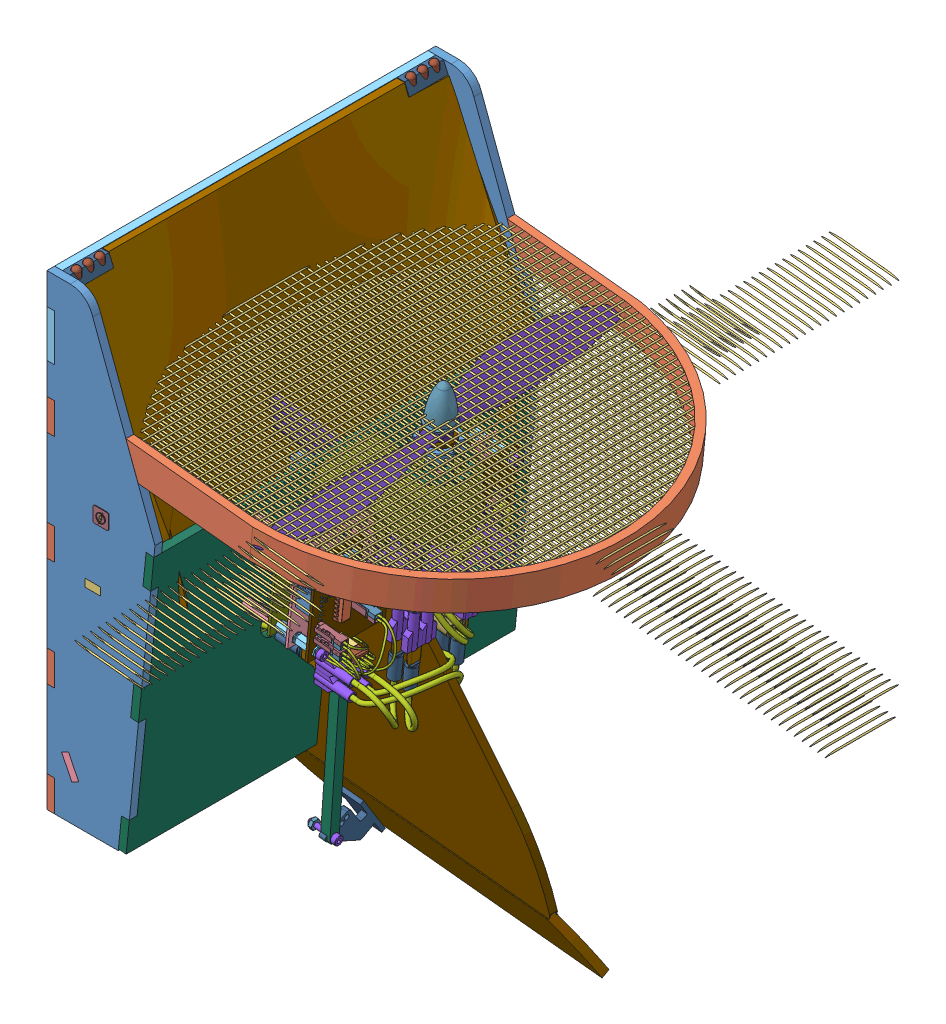
SolidWorks assembly AssTotaleSimu, configuration Défaut. Lengths in mm. (continued)
Components (placement in the parent): (continued)
- AssStructSimu-1: AssStructSimu [Défaut] at (-125.7658 -1.8483 624.6548) x (1 0 0) z (0 0 -1) size (323.53 326.04 251.6) (continued)
  - AssProtec-1: AssProtec [Défaut] at (86.6746 190.4649 284.6351) x (0 0 -1) z (0.101852 -0.9948 0) size (250 237.46 20) (continued)
    - AssGrillage-2: AssGrillage [Défaut] at (339.6086 -132.5428 241.6839) x (0 0 1) z (-1 0 0) size (2.02 237.05 250) (continued)
      - barreau-208: barreau [Défaut] at (-0.1839 -1.5314 233.7823) x (0.998922 0 0.04641) z (0 1 0) size (1 1 400)
      - barreau-209: barreau [Défaut] at (-0.1839 -1.5314 228.7823) x (0.998922 0 0.04641) z (0 1 0) size (1 1 400)
      - barreau-210: barreau [Défaut] at (-0.1839 -1.5314 223.7823) x (0.998922 0 0.04641) z (0 1 0) size (1 1 400)
      - barreau-211: barreau [Défaut] at (-0.1839 -1.5314 218.7823) x (0.998922 0 0.04641) z (0 1 0) size (1 1 400)
      - barreau-212: barreau [Défaut] at (-0.1839 -1.5314 213.7823) x (0.998922 0 0.04641) z (0 1 0) size (1 1 400)
      - barreau-213: barreau [Défaut] at (-0.1839 -1.5314 208.7823) x (0.998922 0 0.04641) z (0 1 0) size (1 1 400)
      - barreau-214: barreau [Défaut] at (-0.1839 -1.5314 203.7823) x (0.998922 0 0.04641) z (0 1 0) size (1 1 400)
  - AssCarte-1: AssCarte [Défaut] at (-42.8534 32.2132 302.028) x (-0.101852 0.9948 0) z (0.9948 0.101852 0) size (91.19 130.57 98.45)
    - carte_onduleur_v4-1: carte_onduleur_v4 [Défaut] at (-25.7639 0.8332 112.9379) size (66.52 130.57 82.34)
      - Layer_1-1: Layer_1 [Défaut] at origin size (60 130 1.61)
      - BTN-1: BTN [Défaut] at (-25.5 7.4 0.803) x (0 -1 0) z (0 0 1) size (6.76 3.64 4.37)
        - Open CASCADE STEP translator 6.8 1.2.1-1: Open CASCADE STEP translator 6.8 1.2.1 [Défaut] at origin size (6.76 3.64 4.37)
          - Body_1-1: Body_1 [Défaut] at (-0.5 -2 0) size (6.76 3.64 4.37)
            - =_[0_1_1_3]-1: =_[0_1_1_3] [Défaut] at origin size (6 3.64 4.37)
            - =_[0_1_1_4]-1: =_[0_1_1_4] [Défaut] at origin size (0.38 1 0.67)
            - =_[0_1_1_5]-1: =_[0_1_1_5] [Défaut] at origin size (0.38 1 0.67)
      - CON_IO1-1: CON_IO1 [Défaut] at (-11.3 12.1 0.803) x (0 -1 0) z (0 0 1) size (16.74 30.7 57.5)
        - Open CASCADE STEP translator 6.8 1.3.1-1: Open CASCADE STEP translator 6.8 1.3.1 [Défaut] at origin size (16.74 30.7 57.5)
          - Body_1_2-1: Body_1_2 [Défaut] at (-3 -15 8) x (0 -1 0) z (-1 0 0) size (30.7 57.5 16.74)
            - 1-1: 1 [Défaut] at origin size (30 50 1.61)
            - 10-1: 10 [Défaut] at (-14.395 31.0465 0.803) x (-1 0 0) z (0 0 1) size (5.59 6.35 1.11)
              - =_[0_1_1_4]-1: =_[0_1_1_4] [Défaut] at origin size (5.59 6.35 1.11)
                - 11-1: 11 [Défaut] at (2 3.3 0) x (-1 0 0) z (0 0 1) size (5.59 6.35 1.11)
                  - =_[0_1_1_3]_2-1: =_[0_1_1_3]_2 [Défaut] at origin size (0.44 0.55 0.36)
                  - =_[0_1_1_4]_2-1: =_[0_1_1_4]_2 [Défaut] at origin size (5.59 4.15 0.36)
                  - =_[0_1_1_5]_2-1: =_[0_1_1_5]_2 [Défaut] at origin size (5.35 6.1 1.1)
                  - =_[0_1_1_6]-1: =_[0_1_1_6] [Défaut] at origin size (0.44 0.55 0.36)
                  - =_[0_1_1_7]-1: =_[0_1_1_7] [Défaut] at origin size (0.44 0.55 0.36)
                  - =_[0_1_1_8]-1: =_[0_1_1_8] [Défaut] at origin size (0.44 0.55 0.36)
            - 13-1: 13 [Défaut] at (-12.62 16.6 -0.803) x (-1 0 0) z (0 0 -1) size (5.59 6.35 1.11)
              - =_[0_1_1_13]-1: =_[0_1_1_13] [Défaut] at origin size (5.59 6.35 1.11)
                - 11-1: 11 [Défaut] at (2 3.3 0) x (-1 0 0) z (0 0 1) size (5.59 6.35 1.11)
                  - =_[0_1_1_3]_2-1: =_[0_1_1_3]_2 [Défaut] at origin size (0.44 0.55 0.36)
                  - =_[0_1_1_4]_2-1: =_[0_1_1_4]_2 [Défaut] at origin size (5.59 4.15 0.36)
                  - =_[0_1_1_5]_2-1: =_[0_1_1_5]_2 [Défaut] at origin size (5.35 6.1 1.1)
                  - =_[0_1_1_6]-1: =_[0_1_1_6] [Défaut] at origin size (0.44 0.55 0.36)
                  - =_[0_1_1_7]-1: =_[0_1_1_7] [Défaut] at origin size (0.44 0.55 0.36)
                  - =_[0_1_1_8]-1: =_[0_1_1_8] [Défaut] at origin size (0.44 0.55 0.36)
            - 16-1: 16 [Défaut] at (-4.2 24.2 0.803) x (-1 0 0) z (0 0 1) size (12.8 0.5 13)
              - =_[0_1_1_15]-1: =_[0_1_1_15] [Défaut] at origin size (12.8 0.5 13)
                - 17-1: 17 [Défaut] at (2.7 0 0) x (1 0 0) z (0 -1 0) size (12.8 13 0.5)
            - 19-1: 19 [Défaut] at (-4.1 6.8 0.803) x (-1 0 0) z (0 0 1) size (12.8 0.5 13)
              - =_[0_1_1_18]-1: =_[0_1_1_18] [Défaut] at origin size (12.8 0.5 13)
                - 17-1: 17 [Défaut] at (2.7 0 0) x (1 0 0) z (0 -1 0) size (12.8 13 0.5)
            - 24-1: 24 [Défaut] at (-8.1 16.5 -0.803) x (0 1 0) z (0 0 -1) size (7.75 5.13 1.17)
              - =_[0_1_1_20]-1: =_[0_1_1_20] [Défaut] at origin size (7.75 5.13 1.17)
                - 20-1: 20 [Défaut] at origin size (7.59 5.13 1.07)
                - 21-1: 21 [Défaut] at (-14.478 0 0) x (-1 0 0) z (0 0 1) size (0.76 5.08 1.17)
                - 22-1: 22 [Défaut] at origin size (0.76 5.08 1.17)
            - 35-1: 35 [Défaut] at (-25.3 25.5 0.803) x (0 -1 0) z (0 0 1) size (6.05 5.2 1.7)
              - =_[0_1_1_25]-1: =_[0_1_1_25] [Défaut] at origin size (6.05 5.2 1.7)
                - 25-1: 25 [Défaut] at origin size (4.3 5.2 1.53)
                - 26-1: 26 [Défaut] at origin size (0.88 0.51 1.06)
                - 27-1: 27 [Défaut] at origin size (0.88 0.51 1.06)
                - 28-1: 28 [Défaut] at origin size (0.88 0.51 1.06)
                - 29-1: 29 [Défaut] at origin size (0.88 0.51 1.06)
                - 30-1: 30 [Défaut] at (11.6 -5.08 0) x (-1 0 0) z (0 0 1) size (0.87 0.51 1.06)
                - 31-1: 31 [Défaut] at (11.6 -2.54 0) x (-1 0 0) z (0 0 1) size (0.87 0.51 1.06)
                - 32-1: 32 [Défaut] at (11.6 0 0) x (-1 0 0) z (0 0 1) size (0.87 0.51 1.06)
                - 33-1: 33 [Défaut] at (11.6 2.54 0) x (-1 0 0) z (0 0 1) size (0.87 0.51 1.06)
            - 40-1: 40 [Défaut] at (-27.6 27.2 0.803) size (2.34 1.04 0.5)
              - =_[0_1_1_36]-1: =_[0_1_1_36] [Défaut] at origin size (2.34 1.04 0.5)
                - 36-1: 36 [Défaut] at origin size (2.29 1.04 0.43)
                - 37-1: 37 [Défaut] at (0.3048 0 0) x (-1 0 0) z (0 0 1) size (0.51 1.02 0.5)
                - 38-1: 38 [Défaut] at origin size (0.51 1.02 0.5)
            - 42-1: 42 [Défaut] at (-22.1 21.6 0.803) x (0 1 0) z (0 0 1) size (2.34 1.04 0.5)
              - =_[0_1_1_36]-1: =_[0_1_1_36] [Défaut] at origin size (2.34 1.04 0.5)
                - 36-1: 36 [Défaut] at origin size (2.29 1.04 0.43)
                - 37-1: 37 [Défaut] at (0.3048 0 0) x (-1 0 0) z (0 0 1) size (0.51 1.02 0.5)
                - 38-1: 38 [Défaut] at origin size (0.51 1.02 0.5)
            - 47-1: 47 [Défaut] at (-14.7664 14.5 -0.803) x (-1 0 0) z (0 0 -1) size (2.34 1.04 0.5)
              - =_[0_1_1_42]-1: =_[0_1_1_42] [Défaut] at origin size (2.34 1.04 0.5)
                - 43-1: 43 [Défaut] at origin size (2.29 1.04 0.43)
                - 44-1: 44 [Défaut] at (0.3048 0 0) x (-1 0 0) z (0 0 1) size (0.51 1.02 0.5)
                - 45-1: 45 [Défaut] at origin size (0.51 1.02 0.5)
            - 57-1: 57 [Défaut] at (-15.3 2.7 -0.803) x (0 -1 0) z (0 0 -1) size (10.36 15.24 6.14)
              - =_[0_1_1_47]-1: =_[0_1_1_47] [Défaut] at origin size (10.36 15.24 6.14)
                - 55-1: 55 [Défaut] at (1.8 -1.2 3) x (1 0 0) z (0 1 0) size (10.36 6.14 15.24)
                  - 54-1: 54 [Défaut] at origin size (10.36 6.14 7.62)
                    - 52-1: 52 [Défaut] at origin size (10.36 6.14 2.54)
                      - 48-1: 48 [Défaut] at origin size (8.4 2.54 2.54)
                      - 49-1: 49 [Défaut] at (-0.0461 1.2682 1.27) x (0 0 -1) z (0.999998 -0.002105 0) size (1.95 5.07 7.58)
                    - 52-2: 52 [Défaut] at (0 0 -2.54) size (10.36 6.14 2.54)
                      - 48-1: 48 [Défaut] at origin size (8.4 2.54 2.54)
                      - 49-1: 49 [Défaut] at (-0.0461 1.2682 1.27) x (0 0 -1) z (0.999998 -0.002105 0) size (1.95 5.07 7.58)
                    - 52-3: 52 [Défaut] at (0 0 -5.08) size (10.36 6.14 2.54)
                      - 48-1: 48 [Défaut] at origin size (8.4 2.54 2.54)
                      - 49-1: 49 [Défaut] at (-0.0461 1.2682 1.27) x (0 0 -1) z (0.999998 -0.002105 0) size (1.95 5.07 7.58)
                  - 54-2: 54 [Défaut] at (0 0 -7.62) size (10.36 6.14 7.62)
                    - 52-1: 52 [Défaut] at origin size (10.36 6.14 2.54)
                      - 48-1: 48 [Défaut] at origin size (8.4 2.54 2.54)
                      - 49-1: 49 [Défaut] at (-0.0461 1.2682 1.27) x (0 0 -1) z (0.999998 -0.002105 0) size (1.95 5.07 7.58)
                    - 52-2: 52 [Défaut] at (0 0 -2.54) size (10.36 6.14 2.54)
                      - 48-1: 48 [Défaut] at origin size (8.4 2.54 2.54)
                      - 49-1: 49 [Défaut] at (-0.0461 1.2682 1.27) x (0 0 -1) z (0.999998 -0.002105 0) size (1.95 5.07 7.58)
                    - 52-3: 52 [Défaut] at (0 0 -5.08) size (10.36 6.14 2.54)
                      - 48-1: 48 [Défaut] at origin size (8.4 2.54 2.54)
                      - 49-1: 49 [Défaut] at (-0.0461 1.2682 1.27) x (0 0 -1) z (0.999998 -0.002105 0) size (1.95 5.07 7.58)
            - 59-1: 59 [Défaut] at (-26.5 31 0.803) x (0 -1 0) z (0 0 1) size (2.34 1.04 0.5)
              - =_[0_1_1_42]-1: =_[0_1_1_42] [Défaut] at origin size (2.34 1.04 0.5)
                - 43-1: 43 [Défaut] at origin size (2.29 1.04 0.43)
                - 44-1: 44 [Défaut] at (0.3048 0 0) x (-1 0 0) z (0 0 1) size (0.51 1.02 0.5)
                - 45-1: 45 [Défaut] at origin size (0.51 1.02 0.5)
            - 61-1: 61 [Défaut] at (-21.6 17.8 0.803) x (-1 0 0) z (0 0 1) size (2.34 1.04 0.5)
              - =_[0_1_1_42]-1: =_[0_1_1_42] [Défaut] at origin size (2.34 1.04 0.5)
                - 43-1: 43 [Défaut] at origin size (2.29 1.04 0.43)
                - 44-1: 44 [Défaut] at (0.3048 0 0) x (-1 0 0) z (0 0 1) size (0.51 1.02 0.5)
                - 45-1: 45 [Défaut] at origin size (0.51 1.02 0.5)
            - 64-1: 64 [Défaut] at (-3.3 17.6 0.803) x (0 -1 0) z (0 0 1) size (8.01 8 14.24)
              - =_[0_1_1_56]-1: =_[0_1_1_56] [Défaut] at origin size (8.01 8 14.24)
                - 62-1: 62 [Défaut] at (1.8 0 0) x (1 0 0) z (0 -1 0) size (8.01 14.24 8)
      - CON_IO2-1: CON_IO2 [Défaut] at (-11.3 -2.7 0.803) x (0 -1 0) z (0 0 1) size (16.74 30.7 57.5)
        - Open CASCADE STEP translator 6.8 1.4.1-1: Open CASCADE STEP translator 6.8 1.4.1 [Défaut] at origin size (16.74 30.7 57.5)
          - Body_1_2-1: Body_1_2 [Défaut] at (-3 -15 8) x (0 -1 0) z (-1 0 0) size (30.7 57.5 16.74)
            - 1-1: 1 [Défaut] at origin size (30 50 1.61)
            - 10-1: 10 [Défaut] at (-14.395 31.0465 0.803) x (-1 0 0) z (0 0 1) size (5.59 6.35 1.11)
              - =_[0_1_1_4]-1: =_[0_1_1_4] [Défaut] at origin size (5.59 6.35 1.11)
                - 11-1: 11 [Défaut] at (2 3.3 0) x (-1 0 0) z (0 0 1) size (5.59 6.35 1.11)
                  - =_[0_1_1_3]_2-1: =_[0_1_1_3]_2 [Défaut] at origin size (0.44 0.55 0.36)
                  - =_[0_1_1_4]_2-1: =_[0_1_1_4]_2 [Défaut] at origin size (5.59 4.15 0.36)
                  - =_[0_1_1_5]_2-1: =_[0_1_1_5]_2 [Défaut] at origin size (5.35 6.1 1.1)
                  - =_[0_1_1_6]-1: =_[0_1_1_6] [Défaut] at origin size (0.44 0.55 0.36)
                  - =_[0_1_1_7]-1: =_[0_1_1_7] [Défaut] at origin size (0.44 0.55 0.36)
                  - =_[0_1_1_8]-1: =_[0_1_1_8] [Défaut] at origin size (0.44 0.55 0.36)
            - 13-1: 13 [Défaut] at (-12.62 16.6 -0.803) x (-1 0 0) z (0 0 -1) size (5.59 6.35 1.11)
              - =_[0_1_1_13]-1: =_[0_1_1_13] [Défaut] at origin size (5.59 6.35 1.11)
                - 11-1: 11 [Défaut] at (2 3.3 0) x (-1 0 0) z (0 0 1) size (5.59 6.35 1.11)
                  - =_[0_1_1_3]_2-1: =_[0_1_1_3]_2 [Défaut] at origin size (0.44 0.55 0.36)
                  - =_[0_1_1_4]_2-1: =_[0_1_1_4]_2 [Défaut] at origin size (5.59 4.15 0.36)
                  - =_[0_1_1_5]_2-1: =_[0_1_1_5]_2 [Défaut] at origin size (5.35 6.1 1.1)
                  - =_[0_1_1_6]-1: =_[0_1_1_6] [Défaut] at origin size (0.44 0.55 0.36)
                  - =_[0_1_1_7]-1: =_[0_1_1_7] [Défaut] at origin size (0.44 0.55 0.36)
                  - =_[0_1_1_8]-1: =_[0_1_1_8] [Défaut] at origin size (0.44 0.55 0.36)
            - 16-1: 16 [Défaut] at (-4.2 24.2 0.803) x (-1 0 0) z (0 0 1) size (12.8 0.5 13)
              - =_[0_1_1_15]-1: =_[0_1_1_15] [Défaut] at origin size (12.8 0.5 13)
                - 17-1: 17 [Défaut] at (2.7 0 0) x (1 0 0) z (0 -1 0) size (12.8 13 0.5)
            - 19-1: 19 [Défaut] at (-4.1 6.8 0.803) x (-1 0 0) z (0 0 1) size (12.8 0.5 13)
              - =_[0_1_1_18]-1: =_[0_1_1_18] [Défaut] at origin size (12.8 0.5 13)
                - 17-1: 17 [Défaut] at (2.7 0 0) x (1 0 0) z (0 -1 0) size (12.8 13 0.5)
            - 24-1: 24 [Défaut] at (-8.1 16.5 -0.803) x (0 1 0) z (0 0 -1) size (7.75 5.13 1.17)
              - =_[0_1_1_20]-1: =_[0_1_1_20] [Défaut] at origin size (7.75 5.13 1.17)
                - 20-1: 20 [Défaut] at origin size (7.59 5.13 1.07)
                - 21-1: 21 [Défaut] at (-14.478 0 0) x (-1 0 0) z (0 0 1) size (0.76 5.08 1.17)
                - 22-1: 22 [Défaut] at origin size (0.76 5.08 1.17)
            - 35-1: 35 [Défaut] at (-25.3 25.5 0.803) x (0 -1 0) z (0 0 1) size (6.05 5.2 1.7)
              - =_[0_1_1_25]-1: =_[0_1_1_25] [Défaut] at origin size (6.05 5.2 1.7)
                - 25-1: 25 [Défaut] at origin size (4.3 5.2 1.53)
                - 26-1: 26 [Défaut] at origin size (0.88 0.51 1.06)
                - 27-1: 27 [Défaut] at origin size (0.88 0.51 1.06)
                - 28-1: 28 [Défaut] at origin size (0.88 0.51 1.06)
                - 29-1: 29 [Défaut] at origin size (0.88 0.51 1.06)
                - 30-1: 30 [Défaut] at (11.6 -5.08 0) x (-1 0 0) z (0 0 1) size (0.87 0.51 1.06)
                - 31-1: 31 [Défaut] at (11.6 -2.54 0) x (-1 0 0) z (0 0 1) size (0.87 0.51 1.06)
                - 32-1: 32 [Défaut] at (11.6 0 0) x (-1 0 0) z (0 0 1) size (0.87 0.51 1.06)
                - 33-1: 33 [Défaut] at (11.6 2.54 0) x (-1 0 0) z (0 0 1) size (0.87 0.51 1.06)
            - 40-1: 40 [Défaut] at (-27.6 27.2 0.803) size (2.34 1.04 0.5)
              - =_[0_1_1_36]-1: =_[0_1_1_36] [Défaut] at origin size (2.34 1.04 0.5)
                - 36-1: 36 [Défaut] at origin size (2.29 1.04 0.43)
                - 37-1: 37 [Défaut] at (0.3048 0 0) x (-1 0 0) z (0 0 1) size (0.51 1.02 0.5)
                - 38-1: 38 [Défaut] at origin size (0.51 1.02 0.5)
            - 42-1: 42 [Défaut] at (-22.1 21.6 0.803) x (0 1 0) z (0 0 1) size (2.34 1.04 0.5)
              - =_[0_1_1_36]-1: =_[0_1_1_36] [Défaut] at origin size (2.34 1.04 0.5)
                - 36-1: 36 [Défaut] at origin size (2.29 1.04 0.43)
                - 37-1: 37 [Défaut] at (0.3048 0 0) x (-1 0 0) z (0 0 1) size (0.51 1.02 0.5)
                - 38-1: 38 [Défaut] at origin size (0.51 1.02 0.5)
            - 47-1: 47 [Défaut] at (-14.7664 14.5 -0.803) x (-1 0 0) z (0 0 -1) size (2.34 1.04 0.5)
              - =_[0_1_1_42]-1: =_[0_1_1_42] [Défaut] at origin size (2.34 1.04 0.5)
                - 43-1: 43 [Défaut] at origin size (2.29 1.04 0.43)
                - 44-1: 44 [Défaut] at (0.3048 0 0) x (-1 0 0) z (0 0 1) size (0.51 1.02 0.5)
                - 45-1: 45 [Défaut] at origin size (0.51 1.02 0.5)
            - 57-1: 57 [Défaut] at (-15.3 2.7 -0.803) x (0 -1 0) z (0 0 -1) size (10.36 15.24 6.14)
              - =_[0_1_1_47]-1: =_[0_1_1_47] [Défaut] at origin size (10.36 15.24 6.14)
                - 55-1: 55 [Défaut] at (1.8 -1.2 3) x (1 0 0) z (0 1 0) size (10.36 6.14 15.24)
                  - 54-1: 54 [Défaut] at origin size (10.36 6.14 7.62)
                    - 52-1: 52 [Défaut] at origin size (10.36 6.14 2.54)
                      - 48-1: 48 [Défaut] at origin size (8.4 2.54 2.54)
                      - 49-1: 49 [Défaut] at (-0.0461 1.2682 1.27) x (0 0 -1) z (0.999998 -0.002105 0) size (1.95 5.07 7.58)
                    - 52-2: 52 [Défaut] at (0 0 -2.54) size (10.36 6.14 2.54)
                      - 48-1: 48 [Défaut] at origin size (8.4 2.54 2.54)
                      - 49-1: 49 [Défaut] at (-0.0461 1.2682 1.27) x (0 0 -1) z (0.999998 -0.002105 0) size (1.95 5.07 7.58)
                    - 52-3: 52 [Défaut] at (0 0 -5.08) size (10.36 6.14 2.54)
                      - 48-1: 48 [Défaut] at origin size (8.4 2.54 2.54)
                      - 49-1: 49 [Défaut] at (-0.0461 1.2682 1.27) x (0 0 -1) z (0.999998 -0.002105 0) size (1.95 5.07 7.58)
                  - 54-2: 54 [Défaut] at (0 0 -7.62) size (10.36 6.14 7.62)
                    - 52-1: 52 [Défaut] at origin size (10.36 6.14 2.54)
                      - 48-1: 48 [Défaut] at origin size (8.4 2.54 2.54)
                      - 49-1: 49 [Défaut] at (-0.0461 1.2682 1.27) x (0 0 -1) z (0.999998 -0.002105 0) size (1.95 5.07 7.58)
                    - 52-2: 52 [Défaut] at (0 0 -2.54) size (10.36 6.14 2.54)
                      - 48-1: 48 [Défaut] at origin size (8.4 2.54 2.54)
                      - 49-1: 49 [Défaut] at (-0.0461 1.2682 1.27) x (0 0 -1) z (0.999998 -0.002105 0) size (1.95 5.07 7.58)
                    - 52-3: 52 [Défaut] at (0 0 -5.08) size (10.36 6.14 2.54)
                      - 48-1: 48 [Défaut] at origin size (8.4 2.54 2.54)
                      - 49-1: 49 [Défaut] at (-0.0461 1.2682 1.27) x (0 0 -1) z (0.999998 -0.002105 0) size (1.95 5.07 7.58)
            - 59-1: 59 [Défaut] at (-26.5 31 0.803) x (0 -1 0) z (0 0 1) size (2.34 1.04 0.5)
              - =_[0_1_1_42]-1: =_[0_1_1_42] [Défaut] at origin size (2.34 1.04 0.5)
                - 43-1: 43 [Défaut] at origin size (2.29 1.04 0.43)
                - 44-1: 44 [Défaut] at (0.3048 0 0) x (-1 0 0) z (0 0 1) size (0.51 1.02 0.5)
                - 45-1: 45 [Défaut] at origin size (0.51 1.02 0.5)
            - 61-1: 61 [Défaut] at (-21.6 17.8 0.803) x (-1 0 0) z (0 0 1) size (2.34 1.04 0.5)
              - =_[0_1_1_42]-1: =_[0_1_1_42] [Défaut] at origin size (2.34 1.04 0.5)
                - 43-1: 43 [Défaut] at origin size (2.29 1.04 0.43)
                - 44-1: 44 [Défaut] at (0.3048 0 0) x (-1 0 0) z (0 0 1) size (0.51 1.02 0.5)
                - 45-1: 45 [Défaut] at origin size (0.51 1.02 0.5)
            - 64-1: 64 [Défaut] at (-3.3 17.6 0.803) x (0 -1 0) z (0 0 1) size (8.01 8 14.24)
              - =_[0_1_1_56]-1: =_[0_1_1_56] [Défaut] at origin size (8.01 8 14.24)
                - 62-1: 62 [Défaut] at (1.8 0 0) x (1 0 0) z (0 -1 0) size (8.01 14.24 8)
      - CON_IO3-1: CON_IO3 [Défaut] at (-11.3 -17.7 0.803) x (0 -1 0) z (0 0 1) size (16.74 30.7 57.5)
        - Open CASCADE STEP translator 6.8 1.5.1-1: Open CASCADE STEP translator 6.8 1.5.1 [Défaut] at origin size (16.74 30.7 57.5)
          - Body_1_2-1: Body_1_2 [Défaut] at (-3 -15 8) x (0 -1 0) z (-1 0 0) size (30.7 57.5 16.74)
            - 1-1: 1 [Défaut] at origin size (30 50 1.61)
            - 10-1: 10 [Défaut] at (-14.395 31.0465 0.803) x (-1 0 0) z (0 0 1) size (5.59 6.35 1.11)
              - =_[0_1_1_4]-1: =_[0_1_1_4] [Défaut] at origin size (5.59 6.35 1.11)
                - 11-1: 11 [Défaut] at (2 3.3 0) x (-1 0 0) z (0 0 1) size (5.59 6.35 1.11)
                  - =_[0_1_1_3]_2-1: =_[0_1_1_3]_2 [Défaut] at origin size (0.44 0.55 0.36)
                  - =_[0_1_1_4]_2-1: =_[0_1_1_4]_2 [Défaut] at origin size (5.59 4.15 0.36)
                  - =_[0_1_1_5]_2-1: =_[0_1_1_5]_2 [Défaut] at origin size (5.35 6.1 1.1)
                  - =_[0_1_1_6]-1: =_[0_1_1_6] [Défaut] at origin size (0.44 0.55 0.36)
                  - =_[0_1_1_7]-1: =_[0_1_1_7] [Défaut] at origin size (0.44 0.55 0.36)
                  - =_[0_1_1_8]-1: =_[0_1_1_8] [Défaut] at origin size (0.44 0.55 0.36)
            - 13-1: 13 [Défaut] at (-12.62 16.6 -0.803) x (-1 0 0) z (0 0 -1) size (5.59 6.35 1.11)
              - =_[0_1_1_13]-1: =_[0_1_1_13] [Défaut] at origin size (5.59 6.35 1.11)
                - 11-1: 11 [Défaut] at (2 3.3 0) x (-1 0 0) z (0 0 1) size (5.59 6.35 1.11)
                  - =_[0_1_1_3]_2-1: =_[0_1_1_3]_2 [Défaut] at origin size (0.44 0.55 0.36)
                  - =_[0_1_1_4]_2-1: =_[0_1_1_4]_2 [Défaut] at origin size (5.59 4.15 0.36)
                  - =_[0_1_1_5]_2-1: =_[0_1_1_5]_2 [Défaut] at origin size (5.35 6.1 1.1)
                  - =_[0_1_1_6]-1: =_[0_1_1_6] [Défaut] at origin size (0.44 0.55 0.36)
                  - =_[0_1_1_7]-1: =_[0_1_1_7] [Défaut] at origin size (0.44 0.55 0.36)
                  - =_[0_1_1_8]-1: =_[0_1_1_8] [Défaut] at origin size (0.44 0.55 0.36)
            - 16-1: 16 [Défaut] at (-4.2 24.2 0.803) x (-1 0 0) z (0 0 1) size (12.8 0.5 13)
              - =_[0_1_1_15]-1: =_[0_1_1_15] [Défaut] at origin size (12.8 0.5 13)
                - 17-1: 17 [Défaut] at (2.7 0 0) x (1 0 0) z (0 -1 0) size (12.8 13 0.5)
            - 19-1: 19 [Défaut] at (-4.1 6.8 0.803) x (-1 0 0) z (0 0 1) size (12.8 0.5 13)
              - =_[0_1_1_18]-1: =_[0_1_1_18] [Défaut] at origin size (12.8 0.5 13)
                - 17-1: 17 [Défaut] at (2.7 0 0) x (1 0 0) z (0 -1 0) size (12.8 13 0.5)
            - 24-1: 24 [Défaut] at (-8.1 16.5 -0.803) x (0 1 0) z (0 0 -1) size (7.75 5.13 1.17)
              - =_[0_1_1_20]-1: =_[0_1_1_20] [Défaut] at origin size (7.75 5.13 1.17)
                - 20-1: 20 [Défaut] at origin size (7.59 5.13 1.07)
                - 21-1: 21 [Défaut] at (-14.478 0 0) x (-1 0 0) z (0 0 1) size (0.76 5.08 1.17)
                - 22-1: 22 [Défaut] at origin size (0.76 5.08 1.17)
            - 35-1: 35 [Défaut] at (-25.3 25.5 0.803) x (0 -1 0) z (0 0 1) size (6.05 5.2 1.7)
              - =_[0_1_1_25]-1: =_[0_1_1_25] [Défaut] at origin size (6.05 5.2 1.7)
                - 25-1: 25 [Défaut] at origin size (4.3 5.2 1.53)
                - 26-1: 26 [Défaut] at origin size (0.88 0.51 1.06)
                - 27-1: 27 [Défaut] at origin size (0.88 0.51 1.06)
                - 28-1: 28 [Défaut] at origin size (0.88 0.51 1.06)
                - 29-1: 29 [Défaut] at origin size (0.88 0.51 1.06)
                - 30-1: 30 [Défaut] at (11.6 -5.08 0) x (-1 0 0) z (0 0 1) size (0.87 0.51 1.06)
                - 31-1: 31 [Défaut] at (11.6 -2.54 0) x (-1 0 0) z (0 0 1) size (0.87 0.51 1.06)
                - 32-1: 32 [Défaut] at (11.6 0 0) x (-1 0 0) z (0 0 1) size (0.87 0.51 1.06)
                - 33-1: 33 [Défaut] at (11.6 2.54 0) x (-1 0 0) z (0 0 1) size (0.87 0.51 1.06)
            - 40-1: 40 [Défaut] at (-27.6 27.2 0.803) size (2.34 1.04 0.5)
              - =_[0_1_1_36]-1: =_[0_1_1_36] [Défaut] at origin size (2.34 1.04 0.5)
                - 36-1: 36 [Défaut] at origin size (2.29 1.04 0.43)
                - 37-1: 37 [Défaut] at (0.3048 0 0) x (-1 0 0) z (0 0 1) size (0.51 1.02 0.5)
                - 38-1: 38 [Défaut] at origin size (0.51 1.02 0.5)
            - 42-1: 42 [Défaut] at (-22.1 21.6 0.803) x (0 1 0) z (0 0 1) size (2.34 1.04 0.5)
              - =_[0_1_1_36]-1: =_[0_1_1_36] [Défaut] at origin size (2.34 1.04 0.5)
                - 36-1: 36 [Défaut] at origin size (2.29 1.04 0.43)
                - 37-1: 37 [Défaut] at (0.3048 0 0) x (-1 0 0) z (0 0 1) size (0.51 1.02 0.5)
                - 38-1: 38 [Défaut] at origin size (0.51 1.02 0.5)
            - 47-1: 47 [Défaut] at (-14.7664 14.5 -0.803) x (-1 0 0) z (0 0 -1) size (2.34 1.04 0.5)
              - =_[0_1_1_42]-1: =_[0_1_1_42] [Défaut] at origin size (2.34 1.04 0.5)
                - 43-1: 43 [Défaut] at origin size (2.29 1.04 0.43)
                - 44-1: 44 [Défaut] at (0.3048 0 0) x (-1 0 0) z (0 0 1) size (0.51 1.02 0.5)
                - 45-1: 45 [Défaut] at origin size (0.51 1.02 0.5)
            - 57-1: 57 [Défaut] at (-15.3 2.7 -0.803) x (0 -1 0) z (0 0 -1) size (10.36 15.24 6.14)
              - =_[0_1_1_47]-1: =_[0_1_1_47] [Défaut] at origin size (10.36 15.24 6.14)
                - 55-1: 55 [Défaut] at (1.8 -1.2 3) x (1 0 0) z (0 1 0) size (10.36 6.14 15.24)
                  - 54-1: 54 [Défaut] at origin size (10.36 6.14 7.62)
                    - 52-1: 52 [Défaut] at origin size (10.36 6.14 2.54)
                      - 48-1: 48 [Défaut] at origin size (8.4 2.54 2.54)
                      - 49-1: 49 [Défaut] at (-0.0461 1.2682 1.27) x (0 0 -1) z (0.999998 -0.002105 0) size (1.95 5.07 7.58)
                    - 52-2: 52 [Défaut] at (0 0 -2.54) size (10.36 6.14 2.54)
                      - 48-1: 48 [Défaut] at origin size (8.4 2.54 2.54)
                      - 49-1: 49 [Défaut] at (-0.0461 1.2682 1.27) x (0 0 -1) z (0.999998 -0.002105 0) size (1.95 5.07 7.58)
                    - 52-3: 52 [Défaut] at (0 0 -5.08) size (10.36 6.14 2.54)
                      - 48-1: 48 [Défaut] at origin size (8.4 2.54 2.54)
                      - 49-1: 49 [Défaut] at (-0.0461 1.2682 1.27) x (0 0 -1) z (0.999998 -0.002105 0) size (1.95 5.07 7.58)
                  - 54-2: 54 [Défaut] at (0 0 -7.62) size (10.36 6.14 7.62)
                    - 52-1: 52 [Défaut] at origin size (10.36 6.14 2.54)
                      - 48-1: 48 [Défaut] at origin size (8.4 2.54 2.54)
                      - 49-1: 49 [Défaut] at (-0.0461 1.2682 1.27) x (0 0 -1) z (0.999998 -0.002105 0) size (1.95 5.07 7.58)
                    - 52-2: 52 [Défaut] at (0 0 -2.54) size (10.36 6.14 2.54)
                      - 48-1: 48 [Défaut] at origin size (8.4 2.54 2.54)
                      - 49-1: 49 [Défaut] at (-0.0461 1.2682 1.27) x (0 0 -1) z (0.999998 -0.002105 0) size (1.95 5.07 7.58)
                    - 52-3: 52 [Défaut] at (0 0 -5.08) size (10.36 6.14 2.54)
                      - 48-1: 48 [Défaut] at origin size (8.4 2.54 2.54)
                      - 49-1: 49 [Défaut] at (-0.0461 1.2682 1.27) x (0 0 -1) z (0.999998 -0.002105 0) size (1.95 5.07 7.58)
            - 59-1: 59 [Défaut] at (-26.5 31 0.803) x (0 -1 0) z (0 0 1) size (2.34 1.04 0.5)
              - =_[0_1_1_42]-1: =_[0_1_1_42] [Défaut] at origin size (2.34 1.04 0.5)
                - 43-1: 43 [Défaut] at origin size (2.29 1.04 0.43)
                - 44-1: 44 [Défaut] at (0.3048 0 0) x (-1 0 0) z (0 0 1) size (0.51 1.02 0.5)
                - 45-1: 45 [Défaut] at origin size (0.51 1.02 0.5)
            - 61-1: 61 [Défaut] at (-21.6 17.8 0.803) x (-1 0 0) z (0 0 1) size (2.34 1.04 0.5)
              - =_[0_1_1_42]-1: =_[0_1_1_42] [Défaut] at origin size (2.34 1.04 0.5)
                - 43-1: 43 [Défaut] at origin size (2.29 1.04 0.43)
                - 44-1: 44 [Défaut] at (0.3048 0 0) x (-1 0 0) z (0 0 1) size (0.51 1.02 0.5)
                - 45-1: 45 [Défaut] at origin size (0.51 1.02 0.5)
            - 64-1: 64 [Défaut] at (-3.3 17.6 0.803) x (0 -1 0) z (0 0 1) size (8.01 8 14.24)
              - =_[0_1_1_56]-1: =_[0_1_1_56] [Défaut] at origin size (8.01 8 14.24)
                - 62-1: 62 [Défaut] at (1.8 0 0) x (1 0 0) z (0 -1 0) size (8.01 14.24 8)
      - C1_1-1: C1_1 [Défaut] at (-20.6336 6.4 -0.803) x (1 0 0) z (0 0 -1) size (2.34 1.04 0.5)
        - Open CASCADE STEP translator 6.8 1.6.1-1: Open CASCADE STEP translator 6.8 1.6.1 [Défaut] at origin size (2.34 1.04 0.5)
          - Body_1-1: Body_1 [Défaut] at origin size (2.29 1.04 0.43)
          - Pin_1-1: Pin_1 [Défaut] at (0.3048 0 0) x (-1 0 0) z (0 0 1) size (0.51 1.02 0.5)
          - Pin_2-1: Pin_2 [Défaut] at origin size (0.51 1.02 0.5)
      - C1_2-1: C1_2 [Défaut] at (-24.2 6.4 -0.803) x (1 0 0) z (0 0 -1) size (2.34 1.04 0.5)
        - Open CASCADE STEP translator 6.8 1.6.1-1: Open CASCADE STEP translator 6.8 1.6.1 [Défaut] at origin size (2.34 1.04 0.5)
          - Body_1-1: Body_1 [Défaut] at origin size (2.29 1.04 0.43)
          - Pin_1-1: Pin_1 [Défaut] at (0.3048 0 0) x (-1 0 0) z (0 0 1) size (0.51 1.02 0.5)
          - Pin_2-1: Pin_2 [Défaut] at origin size (0.51 1.02 0.5)
      - C_F-1: C_F [Défaut] at (-16.2432 4.45 -0.803) x (0 -1 0) z (0 0 -1) size (2.34 1.04 0.5)
        - Open CASCADE STEP translator 6.8 1.6.1-1: Open CASCADE STEP translator 6.8 1.6.1 [Défaut] at origin size (2.34 1.04 0.5)
          - Body_1-1: Body_1 [Défaut] at origin size (2.29 1.04 0.43)
          - Pin_1-1: Pin_1 [Défaut] at (0.3048 0 0) x (-1 0 0) z (0 0 1) size (0.51 1.02 0.5)
          - Pin_2-1: Pin_2 [Défaut] at origin size (0.51 1.02 0.5)
      - D_LED_STATE1-1: D_LED_STATE1 [Défaut] at (-6.8906 -21.6 0.803) size (2.34 1.04 0.5)
        - Open CASCADE STEP translator 6.8 1.6.1-1: Open CASCADE STEP translator 6.8 1.6.1 [Défaut] at origin size (2.34 1.04 0.5)
          - Body_1-1: Body_1 [Défaut] at origin size (2.29 1.04 0.43)
          - Pin_1-1: Pin_1 [Défaut] at (0.3048 0 0) x (-1 0 0) z (0 0 1) size (0.51 1.02 0.5)
          - Pin_2-1: Pin_2 [Défaut] at origin size (0.51 1.02 0.5)
      - PICKIT-1: PICKIT [Défaut] at (-24.1 -30.5 0.803) size (15.24 5 14.3)
        - Open CASCADE STEP translator 6.8 1.10.1-1: Open CASCADE STEP translator 6.8 1.10.1 [Défaut] at origin size (15.24 5 14.3)
          - Body_1_2-1: Body_1_2 [Défaut] at (6.3 0 12) size (15.24 5 14.3)
      - C_DEC_CUR-1: C_DEC_CUR [Défaut] at (-8.9496 5.7572 -0.803) x (0 1 0) z (0 0 -1) size (2.34 1.04 0.5)
        - Open CASCADE STEP translator 6.8 1.6.1-1: Open CASCADE STEP translator 6.8 1.6.1 [Défaut] at origin size (2.34 1.04 0.5)
          - Body_1-1: Body_1 [Défaut] at origin size (2.29 1.04 0.43)
          - Pin_1-1: Pin_1 [Défaut] at (0.3048 0 0) x (-1 0 0) z (0 0 1) size (0.51 1.02 0.5)
          - Pin_2-1: Pin_2 [Défaut] at origin size (0.51 1.02 0.5)
      - R_F-1: R_F [Défaut] at (-14.65 4.4432 -0.803) x (0 -1 0) z (0 0 -1) size (2.34 1.04 0.5)
        - Open CASCADE STEP translator 6.8 1.12.1-1: Open CASCADE STEP translator 6.8 1.12.1 [Défaut] at origin size (2.34 1.04 0.5)
          - Body_1_3-1: Body_1_3 [Défaut] at origin size (2.29 1.04 0.43)
          - Pin_1_2-1: Pin_1_2 [Défaut] at (0.3048 0 0) x (-1 0 0) z (0 0 1) size (0.51 1.02 0.5)
          - Pin_2_2-1: Pin_2_2 [Défaut] at origin size (0.51 1.02 0.5)
      - R_GAIN1-1: R_GAIN1 [Défaut] at (-13.95 5.7568 -0.803) x (0 1 0) z (0 0 -1) size (2.34 1.04 0.5)
        - Open CASCADE STEP translator 6.8 1.12.1-1: Open CASCADE STEP translator 6.8 1.12.1 [Défaut] at origin size (2.34 1.04 0.5)
          - Body_1_3-1: Body_1_3 [Défaut] at origin size (2.29 1.04 0.43)
          - Pin_1_2-1: Pin_1_2 [Défaut] at (0.3048 0 0) x (-1 0 0) z (0 0 1) size (0.51 1.02 0.5)
          - Pin_2_2-1: Pin_2_2 [Défaut] at origin size (0.51 1.02 0.5)
      - R_GAIN2-1: R_GAIN2 [Défaut] at (-15.65 7.9176 -0.803) x (0 -1 0) z (0 0 -1) size (2.34 1.04 0.5)
        - Open CASCADE STEP translator 6.8 1.12.1-1: Open CASCADE STEP translator 6.8 1.12.1 [Défaut] at origin size (2.34 1.04 0.5)
          - Body_1_3-1: Body_1_3 [Défaut] at origin size (2.29 1.04 0.43)
          - Pin_1_2-1: Pin_1_2 [Défaut] at (0.3048 0 0) x (-1 0 0) z (0 0 1) size (0.51 1.02 0.5)
          - Pin_2_2-1: Pin_2_2 [Défaut] at origin size (0.51 1.02 0.5)
      - R_LED_STATE1-1: R_LED_STATE1 [Défaut] at (-6.9242 -19.9 0.803) size (2.34 1.04 0.5)
        - Open CASCADE STEP translator 6.8 1.12.1-1: Open CASCADE STEP translator 6.8 1.12.1 [Défaut] at origin size (2.34 1.04 0.5)
          - Body_1_3-1: Body_1_3 [Défaut] at origin size (2.29 1.04 0.43)
          - Pin_1_2-1: Pin_1_2 [Défaut] at (0.3048 0 0) x (-1 0 0) z (0 0 1) size (0.51 1.02 0.5)
          - Pin_2_2-1: Pin_2_2 [Défaut] at origin size (0.51 1.02 0.5)
      - R_RESET1-1: R_RESET1 [Défaut] at (-23 7.9 0.803) size (2.34 1.04 0.5)
        - Open CASCADE STEP translator 6.8 1.12.1-1: Open CASCADE STEP translator 6.8 1.12.1 [Défaut] at origin size (2.34 1.04 0.5)
          - Body_1_3-1: Body_1_3 [Défaut] at origin size (2.29 1.04 0.43)
          - Pin_1_2-1: Pin_1_2 [Défaut] at (0.3048 0 0) x (-1 0 0) z (0 0 1) size (0.51 1.02 0.5)
          - Pin_2_2-1: Pin_2_2 [Défaut] at origin size (0.51 1.02 0.5)
      - U_DSPIC-1: U_DSPIC [Défaut] at (1.863 -2.61 0.803) size (7.92 35.56 7.75)
        - Open CASCADE STEP translator 6.8 1.17.1-1: Open CASCADE STEP translator 6.8 1.17.1 [Défaut] at origin size (7.92 35.56 7.75)
          - Body_1_4-1: Body_1_4 [Défaut] at (0 -0.2 4) x (1 0 0) z (0 -1 0) size (7.92 7.75 35.56)
      - C_DEC_DSPIC-1: C_DEC_DSPIC [Défaut] at (7.7 -8.8 -0.803) x (0 1 0) z (0 0 -1) size (2.34 1.04 0.5)
        - Open CASCADE STEP translator 6.8 1.6.1-1: Open CASCADE STEP translator 6.8 1.6.1 [Défaut] at origin size (2.34 1.04 0.5)
          - Body_1-1: Body_1 [Défaut] at origin size (2.29 1.04 0.43)
          - Pin_1-1: Pin_1 [Défaut] at (0.3048 0 0) x (-1 0 0) z (0 0 1) size (0.51 1.02 0.5)
          - Pin_2-1: Pin_2 [Défaut] at origin size (0.51 1.02 0.5)
      - IN-1: IN [Défaut] at (24.3 -5.3 0.803) x (0 1 0) z (0 0 1) size (10.21 15.56 26.9)
        - Open CASCADE STEP translator 6.8 1.19.1-1: Open CASCADE STEP translator 6.8 1.19.1 [Défaut] at origin size (10.21 15.56 26.9)
          - Body_1_3-1: Body_1_3 [Défaut] at (-13.5 1.8 3) x (0 1 0) z (1 0 0) size (15.56 26.9 10.21)
            - Imported-1: Imported [Défaut] at (2.0451 -4.5908 20.9802) size (8.6 15.9 10.16)
            - Imported-2: Imported [Défaut] at (-1.6683 9.1092 15.9802) x (0 0 1) z (-1 0 0) size (10.1 18.2 15.1)
              - Imported_2-1: Imported_2 [Défaut] at origin size (10.1 18.2 15.1)
              - Imported_3-1: Imported_3 [Défaut] at origin size (3.43 12.4 4.99)
              - Imported_4-1: Imported_4 [Défaut] at origin size (3.43 12.4 4.99)
              - Imported_5-1: Imported_5 [Défaut] at origin size (3.9 4.9 7)
              - Imported_6-1: Imported_6 [Défaut] at origin size (3.9 4.9 7)
              - Imported_7-1: Imported_7 [Défaut] at origin size (3.8 3.8 6.92)
              - Imported_8-1: Imported_8 [Défaut] at origin size (3.8 3.8 6.92)
              - Imported_9-1: Imported_9 [Défaut] at origin size (9 2.4 14.2)
      - CARTE_CMD-1: CARTE_CMD [Défaut] at (25 57.2 0.803) size (60.1 130 26.71)
        - Open CASCADE STEP translator 6.8 1.20.1-1: Open CASCADE STEP translator 6.8 1.20.1 [Défaut] at origin size (60.1 130 26.71)
          - Body_1_4-1: Body_1_4 [Défaut] at (-55 5 12) size (60.1 130 26.71)
            - 1_2-1: 1_2 [Défaut] at origin size (60.1 130 1.61)
            - 4-1: 4 [Défaut] at (23.6 -124.9 0.803) x (0 1 0) z (0 0 1) size (5 15.24 14.3)
              - =_[0_1_1_4]_2-1: =_[0_1_1_4]_2 [Défaut] at origin size (5 15.24 14.3)
                - 5-1: 5 [Défaut] at (0 -6.5 -13) x (0 1 0) z (0 0 -1) size (15.24 5 14.3)
            - 7-1: 7 [Défaut] at (23.6 -5 0.803) x (0 1 0) z (0 0 1) size (5 15.24 14.3)
              - =_[0_1_1_7]-1: =_[0_1_1_7] [Défaut] at origin size (5 15.24 14.3)
                - 5-1: 5 [Défaut] at (0 -6.5 -13) x (0 1 0) z (0 0 -1) size (15.24 5 14.3)
            - 10_2-1: 10_2 [Défaut] at (18.4 -115.6 0.803) size (25.4 7.92 7.75)
              - =_[0_1_1_9]-1: =_[0_1_1_9] [Défaut] at origin size (25.4 7.92 7.75)
                - 8-1: 8 [Défaut] at (11.2 4 0) x (0 1 0) z (1 0 0) size (7.92 7.75 25.4)
            - 13_2-1: 13_2 [Défaut] at (55.4 -114.7 0.803) x (-1 0 0) z (0 0 1) size (5 7.62 14.3)
              - =_[0_1_1_12]-1: =_[0_1_1_12] [Défaut] at origin size (5 7.62 14.3)
                - 11-1: 11 [Défaut] at (0 -2.5 11) x (0 -1 0) z (0 0 1) size (7.62 5 14.3)
            - 25-1: 25 [Défaut] at (56.9 -12.8 0.803) x (-1 0 0) z (0 0 1) size (16.02 47.26 11.05)
              - =_[0_1_1_15]_2-1: =_[0_1_1_15]_2 [Défaut] at origin size (16.02 47.26 11.05)
                - 23-1: 23 [Défaut] at (-36.5 21 4) x (0 -1 0) z (1 0 0) size (47.26 11.05 16.02)
                  - 14-1: 14 [Défaut] at (-7.4961 -1.5352 42.5833) size (42.58 6.55 16.01)
                  - 22-1: 22 [Défaut] at (19.3039 2.3748 37.905) x (-1 0 0) z (0 0 -1) size (10.36 6.14 15.24)
                    - 21-1: 21 [Défaut] at origin size (10.36 6.14 7.62)
                      - 19_2-1: 19_2 [Défaut] at origin size (10.36 6.14 2.54)
                        - 15-1: 15 [Défaut] at origin size (8.4 2.54 2.54)
                        - 16-1: 16 [Défaut] at (-0.0461 1.2682 1.27) x (0 0 -1) z (0.999998 -0.002105 0) size (1.95 5.07 7.58)
                      - 19_2-2: 19_2 [Défaut] at (0 0 -2.54) size (10.36 6.14 2.54)
                        - 15-1: 15 [Défaut] at origin size (8.4 2.54 2.54)
                        - 16-1: 16 [Défaut] at (-0.0461 1.2682 1.27) x (0 0 -1) z (0.999998 -0.002105 0) size (1.95 5.07 7.58)
                      - 19_2-3: 19_2 [Défaut] at (0 0 -5.08) size (10.36 6.14 2.54)
                        - 15-1: 15 [Défaut] at origin size (8.4 2.54 2.54)
                        - 16-1: 16 [Défaut] at (-0.0461 1.2682 1.27) x (0 0 -1) z (0.999998 -0.002105 0) size (1.95 5.07 7.58)
                    - 21-2: 21 [Défaut] at (0 0 -7.62) size (10.36 6.14 7.62)
                      - 19_2-1: 19_2 [Défaut] at origin size (10.36 6.14 2.54)
                        - 15-1: 15 [Défaut] at origin size (8.4 2.54 2.54)
                        - 16-1: 16 [Défaut] at (-0.0461 1.2682 1.27) x (0 0 -1) z (0.999998 -0.002105 0) size (1.95 5.07 7.58)
                      - 19_2-2: 19_2 [Défaut] at (0 0 -2.54) size (10.36 6.14 2.54)
                        - 15-1: 15 [Défaut] at origin size (8.4 2.54 2.54)
                        - 16-1: 16 [Défaut] at (-0.0461 1.2682 1.27) x (0 0 -1) z (0.999998 -0.002105 0) size (1.95 5.07 7.58)
                      - 19_2-3: 19_2 [Défaut] at (0 0 -5.08) size (10.36 6.14 2.54)
                        - 15-1: 15 [Défaut] at origin size (8.4 2.54 2.54)
                        - 16-1: 16 [Défaut] at (-0.0461 1.2682 1.27) x (0 0 -1) z (0.999998 -0.002105 0) size (1.95 5.07 7.58)
            - 31-1: 31 [Défaut] at (12.9 -104.5 0.803) size (6.76 3.64 4.37)
              - =_[0_1_1_24]-1: =_[0_1_1_24] [Défaut] at origin size (6.76 3.64 4.37)
                - 29-1: 29 [Défaut] at (-0.3 -2 0) size (6.76 3.64 4.37)
                  - =_[0_1_1_3]_3-1: =_[0_1_1_3]_3 [Défaut] at origin size (6 3.64 4.37)
                  - =_[0_1_1_4]_3-1: =_[0_1_1_4]_3 [Défaut] at origin size (0.38 1 0.67)
                  - =_[0_1_1_5]_3-1: =_[0_1_1_5]_3 [Défaut] at origin size (0.38 1 0.67)
            - 36-1: 36 [Défaut] at (28.6 -12.2 0.803) x (0 -1 0) z (0 0 1) size (2.34 1.04 0.5)
              - =_[0_1_1_30]-1: =_[0_1_1_30] [Défaut] at origin size (2.34 1.04 0.5)
                - 32_2-1: 32_2 [Défaut] at origin size (2.29 1.04 0.43)
                - 33_2-1: 33_2 [Défaut] at (0.3048 0 0) x (-1 0 0) z (0 0 1) size (0.51 1.02 0.5)
                - 34-1: 34 [Défaut] at origin size (0.51 1.02 0.5)
            - 38-1: 38 [Défaut] at (23.7 -12.2 0.803) x (0 -1 0) z (0 0 1) size (2.34 1.04 0.5)
              - =_[0_1_1_30]-1: =_[0_1_1_30] [Défaut] at origin size (2.34 1.04 0.5)
                - 32_2-1: 32_2 [Défaut] at origin size (2.29 1.04 0.43)
                - 33_2-1: 33_2 [Défaut] at (0.3048 0 0) x (-1 0 0) z (0 0 1) size (0.51 1.02 0.5)
                - 34-1: 34 [Défaut] at origin size (0.51 1.02 0.5)
            - 40_2-1: 40_2 [Défaut] at (26.2 -12.2 0.803) x (0 -1 0) z (0 0 1) size (2.34 1.04 0.5)
              - =_[0_1_1_30]-1: =_[0_1_1_30] [Défaut] at origin size (2.34 1.04 0.5)
                - 32_2-1: 32_2 [Défaut] at origin size (2.29 1.04 0.43)
